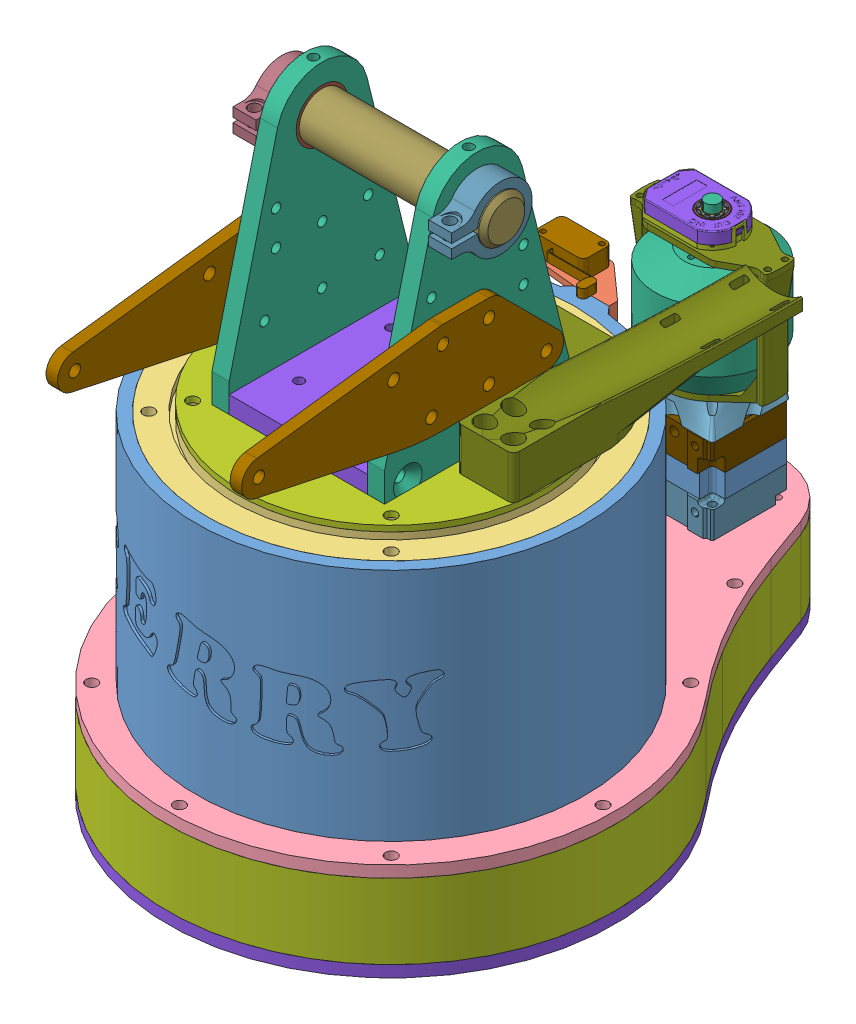
SolidWorks assembly Base, configuration Default. Lengths in mm.
Overall size (246.45 331.62 351.82).
89 component instances, 60 part files, 28 mates.
Components (placement in the parent):
- BotTurretHousing^Base-1: BotTurretHousing^Base [Default] at origin size (214.7 129.6 217.88) (virtual)
- SwitchTripper^Base-2: SwitchTripper^Base [Default] at origin size (28.57 11.52 54.14) (hidden, virtual)
- J1SwitchMount^Base-1: J1SwitchMount^Base [Default] at origin size (48.43 36.2 22.29) (virtual)
- 8in-1: 8in [Default] at (0 58.8 0) size (202 16 202)
- 8in-2: 8in [Default] at (0 -58.8 0) x (1 0 0) z (0 0 -1) size (202 16 202)
- BasePlate^Base-1: BasePlate^Base [Default] at origin size (246.45 6.35 338.52) (virtual)
- BotTurretPlate^Base-1: BotTurretPlate^Base [Default] at origin size (168.46 3.17 168.46) (virtual)
- SideTurretPlate^Base-1: SideTurretPlate^Base [Default] at origin size (9.52 279.65 102.6) (virtual)
- SideTurretPlate^Base-3: SideTurretPlate^Base [Default] x (-1 0 0) z (0 0 -1) size (9.52 279.65 102.6) (virtual)
- TopTurretPlate^Base-1: TopTurretPlate^Base [Default] at origin size (168.46 3.17 168.46) (virtual)
- TopBrace-1: TopBrace [Default] at origin size (76.2 9.53 102.6)
- PivotPlate^Base-1: PivotPlate^Base [Default] at origin size (6.35 50.8 177.8) (virtual)
- PivotPlate^Base-2: PivotPlate^Base [Default] at (101.6 0 0) size (6.35 50.8 177.8) (virtual)
- Keda9to1-1: Keda9to1 [Default] at (0 -48.175 -154.975) x (0 -1 0) z (1 0 0) size (176.96 63 76.93)
  - VersaPlanetary_v2_Single_Stage_10_1_with_BAG.STEP-1: VersaPlanetary_v2_Single_Stage_10_1_with_BAG.STEP [Default] at origin size (163.4 63.52 63.52)
    - 217-2820 Rev1_Public.STEP-1: 217-2820 Rev1_Public.STEP [Default] at (-4.6546 22.225 0) x (0 -0.456494 0.889726) z (-1 0 0) size (39.22 38.88 17.4)
      - 217-2625-100.STEP-1: 217-2625-100.STEP [Default] at origin size (39.22 38.88 12.7)
        - 217-2625-008 Rev1.STEP-1: 217-2625-008 Rev1.STEP [Default] at origin size (34.7 34.7 4.7)
        - 217-2625-010 Rev1.STEP-1: 217-2625-010 Rev1.STEP [Default] at (0 10.193 3.65) x (0.999813 0.019336 0) z (0 0 1) size (4 4 12)
        - 217-2625-010 Rev1.STEP-2: 217-2625-010 Rev1.STEP [Default] at (8.691 -5.3258 3.65) size (4 4 12)
        - 217-2625-010 Rev1.STEP-3: 217-2625-010 Rev1.STEP [Default] at (-8.691 -5.3258 3.65) size (4 4 12)
        - 217-2625-005 Rev1_Planet_Revolving_Follower01.STEP-1: 217-2625-005 Rev1_Planet_Revolving_Follower01.STEP [Default] at (8.691 -5.3258 6.35) x (0.932816 0.360354 0) z (0 0 1) size (16.89 16.89 8)
        - 217-2625-005 Rev1_Planet_Revolving_Follower01.STEP-2: 217-2625-005 Rev1_Planet_Revolving_Follower01.STEP [Default] at (-8.691 -5.3258 6.35) x (-0.932788 -0.360426 0) z (0 0 1) size (16.89 16.89 8)
        - 217-2625-005 Rev1_Planet_Revolving_Follower01.STEP-3: 217-2625-005 Rev1_Planet_Revolving_Follower01.STEP [Default] at (0 10.193 6.35) x (0.893583 0.448898 0) z (0 0 1) size (16.89 16.89 8)
      - 217-2625-007 Rev1_Public.STEP-1: 217-2625-007 Rev1_Public.STEP [Default] at (0 0 6.7) x (0.992772 0.120019 0) z (0 0 1) size (15.27 15.27 12.7)
    - 217-2625-026 Rev1.STEP-1: 217-2625-026 Rev1.STEP [Default] at (-6.5 22.225 0) x (0 -1 0) z (-1 0 0) size (44.45 42 18.12)
    - 217-2742-001 Rev4.STEP-1: 217-2742-001 Rev4.STEP [Default] at (0.2002 22.225 0) x (1 0 0) z (0 -0.092627 0.995701) size (7 28 28)
    - 217-2742-001 Rev4.STEP-2: 217-2742-001 Rev4.STEP [Default] at (8.2002 22.225 0) size (7 28 28)
    - 217-2625-017 Rev1_9714K61.STEP-1: 217-2625-017 Rev1_9714K61.STEP [Default] at (7.42 22.3002 -0.342) x (0 0.56703 0.823697) z (0 -0.823697 0.56703) size (28.51 4.98 27.43)
    - 217-2625-003 Rev1.STEP-1: 217-2625-003 Rev1.STEP [Default] at (7.4478 22.225 0) x (0 -1 0) z (1 0 0) size (17 17 64.11) (hidden)
    - 217-2625-018 Rev1_98541A410.STEP-1: 217-2625-018 Rev1_98541A410.STEP [Default] at (-0.7046 22.225 0) x (1 0 0) z (0 -0.017452 0.999848) size (1 19.6 17.4)
    - 832-1750-Ring-Gear-Screw_SSA0832-0500ZC.STEP-1: 832-1750-Ring-Gear-Screw_SSA0832-0500ZC.STEP [Default] at (-30.7 4.725 -17.5) x (0 0.997447 0.071411) z (0 -0.071411 0.997447) size (6.73 48.51 6.73) (hidden)
    - 832-1750-Ring-Gear-Screw_SSA0832-0500ZC.STEP-2: 832-1750-Ring-Gear-Screw_SSA0832-0500ZC.STEP [Default] at (-30.7 39.725 17.5) x (0 0.005929 0.999982) z (0 -0.999982 0.005929) size (6.73 48.51 6.73) (hidden)
    - 217-2625-025 Rev1.STEP-1: 217-2625-025 Rev1.STEP [Default] at (-23.2 22.225 0) x (0 -1 0) z (-1 0 0) size (44.45 42 18)
    - 217-4649-002 Rev1_SSA0832-0500ZC.STEP-1: 217-4649-002 Rev1_SSA0832-0500ZC.STEP [Default] at (-33.7 4.2645 17.9605) x (0 0.33842 -0.940995) z (0 0.940995 0.33842) size (6.73 16.76 6.73) (hidden)
    - 217-4649-002 Rev1_SSA0832-0500ZC.STEP-2: 217-4649-002 Rev1_SSA0832-0500ZC.STEP [Default] at (-33.7 40.1855 -17.9605) x (0 -0.308932 -0.951084) z (0 0.951084 -0.308932) size (6.73 16.76 6.73) (hidden)
    - 217-4649-006 Rev1_SSA0004-008BA.STEP-1: 217-4649-006 Rev1_SSA0004-008BA.STEP [Default] at (-30.7 22.225 12.5) x (0 0.5 -0.866025) z (0 -0.866025 -0.5) size (7 14 7) (hidden)
    - 217-4649-006 Rev1_SSA0004-008BA.STEP-2: 217-4649-006 Rev1_SSA0004-008BA.STEP [Default] at (-30.7 22.225 -12.5) x (0 -0.5 0.866025) z (0 0.866025 0.5) size (7 14 7) (hidden)
    - 217-2822-003 Rev4.STEP-1: 217-2822-003 Rev4.STEP [Default] at (-32.2 22.225 0) x (0 -1 0) z (-1 0 0) size (42 42 4.8) (hidden)
    - 217-3351 Rev2.STEP-1: 217-3351 Rev2.STEP [Default] at (-33.7 22.225 0) x (0 0 1) z (1 0 0) size (59.07 59.07 84.5) (hidden)
    - 217-2816-001 Rev1.STEP-1: 217-2816-001 Rev1.STEP [Default] at (-6.35 22.225 0) x (0 -1 0) z (1 0 0) size (42 42 14.51)
    - 217-4649-001 Rev1.STEP-1: 217-4649-001 Rev1.STEP [Default] at (-20.046 22.225 0) x (0 -1 0) z (1 0 0) size (18 18 13)
    - 217-4649-007 Rev1_94105A824.STEP-1: 217-4649-007 Rev1_94105A824.STEP [Default] at (-25.521 22.225 -6.7835) x (-0.996104 -0.088191 0) z (0 0 -1) size (4.83 4.83 4.77)
    - 217-2625-011 Rev1.STEP-1: 217-2625-011 Rev1.STEP [Default] at (-24.7818 22.225 0) x (0 0 1) z (0 -1 0) size (8.01 7.5 7.94) (hidden)
  - VersaPlanetary_CIM_Motor_Output_Shaft_Kit_217-2893-1: VersaPlanetary_CIM_Motor_Output_Shaft_Kit_217-2893 [Default] at (7.4478 22.225 0) x (0 0 -1) z (1 0 0) size (17 17 57.85)
  - KedaAdapter^Keda9to1-1: KedaAdapter^Keda9to1 [Default] at origin size (17.82 53.01 53.01) (virtual)
  - 192kvMotorEncoded-1: 192kvMotorEncoded [Default] at (-51.0318 22.225 0) x (0 -1 0) z (0 0 -1) size (63 104.52 76.93)
    - BetterKEDA-1: BetterKEDA [Default] at origin size (63 104.52 63)
    - CUI_DEVICES_AMT102-0048-N2000-S-1: CUI_DEVICES_AMT102-0048-N2000-S [Default] at (0 65.12 0) x (1 0 0) z (0 1 0) size (36.33 46.21 9.2)
      - CUI_DEVICES_AMT102-0048-N2000-S.step-1: CUI_DEVICES_AMT102-0048-N2000-S.step [Default] at origin size (36.33 46.21 9.2)
        - AMT-102-Base-REV-K.step-1: AMT-102-Base-REV-K.step [Default] x (-1 0 0) z (0 0 -1) size (28.78 43.39 9.06)
        - AMT-102-Top-Cover-REV-H.step-1: AMT-102-Top-Cover-REV-H.step [Default] at (0 0 5.23) x (-1 0 0) z (0 0 -1) size (28.6 43.26 6.55)
        - AMT-Sleeve-REV-D_ 2 mm.step-1: AMT-Sleeve-REV-D_ 2 mm.step [Default] at (0 0 -2.42) x (0.999996 0.002864 0) z (0 0 1) size (10.79 10.79 7.8)
        - AMT-Hub-Top-REV-D1.step-1: AMT-Hub-Top-REV-D1.step [Default] at (0 0 2.13) x (0.999996 0.002864 0) z (0 0 1) size (14 14 5.67)
        - AMT-Hub-Bottom-REV-B.step-1: AMT-Hub-Bottom-REV-B.step [Default] at (0 0 2.43) x (0.999998 -0.001942 0) z (0 0 1) size (17.3 17.3 3.2)
        - AMT10X-Shaft-Adaptor-REV-E.step-1: AMT10X-Shaft-Adaptor-REV-E.step [Default] at (0 0 0.03) x (0.999996 0.002864 0) z (0 0 1) size (11.8 11.8 7.8)
        - Receiver-board.step-1: Receiver-board.step [Default] at (72.2834 -20.351 3.03) x (-1 0 0) z (0 0 -1) size (26.5 26.62 0.41)
        - Rotor-board-REV F.step-1: Rotor-board-REV F.step [Default] at (0 0 2.13) x (0.807874 -0.589355 0) z (0 0 1) size (26 26 0.3)
        - Transmitter-board AMT10_AMT-102.step-1: Transmitter-board AMT10_AMT-102.step [Default] at (19.1596 -17.1102 1.22) x (-1 0 0) z (0 0 -1) size (26.63 38.43 4.41)
    - Body^192kvMotorEncoded-1: Body^192kvMotorEncoded [Default] at origin size (53 64.53 76.93) (virtual)
- J1Pulley-1: J1Pulley [Default] at (0 -97.675 0) size (144.9 27.7 144.9)
- 15Tpulley-2: 15Tpulley [Default] at (0 -89.675 -177.2) size (28 28 28)
- J1Belt133T^Base-1: J1Belt133T^Base [Default] at origin size (148.26 15.01 264.1) (virtual)
- TensionPillarJ1-1: TensionPillarJ1 [Default] at (5.0959 -8.1275 -9.5995) size (38.1 25.73 38.1)
  - 98019A228_MIL SPEC. 300 SERIES SS FLAT WASHER-1: 98019A228_MIL SPEC. 300 SERIES SS FLAT WASHER [98019A228] at (20.3041 -73.2587 -110.4505) x (0.972939 0 -0.231063) z (0.231063 0 0.972939) size (9.53 0.71 9.53)
  - 60355K701_BALL BEARING-1: 60355K701_BALL BEARING [60355K701] at (20.3041 -75.7479 -110.4505) x (1 0 0) z (0 1 0) size (15.88 15.88 4.98)
  - Roller^TensionPillarJ1-1: Roller^TensionPillarJ1 [Default] at (-2.0675 -15.5777 2.6827) size (38.1 15 38.1) (virtual)
  - 60355K701_BALL BEARING-2: 60355K701_BALL BEARING [60355K701] at (20.3041 -86.2673 -110.4505) x (1 0 0) z (0 1 0) size (15.88 15.88 4.98)
  - 375spacer-1: 375spacer [92510A777] at (20.3041 -67.785 -110.4505) x (1 0 0) z (0 -1 0) size (15.88 15.88 9.53)
- TensionPillarJ1-2: TensionPillarJ1 [Default] at (-5.0959 -8.1275 -230.5005) x (-1 0 0) z (0 0 -1) size (38.1 25.73 38.1)
  - 98019A228_MIL SPEC. 300 SERIES SS FLAT WASHER-1: 98019A228_MIL SPEC. 300 SERIES SS FLAT WASHER [98019A228] at (20.3041 -73.2587 -110.4505) x (0.972939 0 -0.231063) z (0.231063 0 0.972939) size (9.53 0.71 9.53)
  - 60355K701_BALL BEARING-1: 60355K701_BALL BEARING [60355K701] at (20.3041 -75.7479 -110.4505) x (1 0 0) z (0 1 0) size (15.88 15.88 4.98)
  - Roller^TensionPillarJ1-1: Roller^TensionPillarJ1 [Default] at (-2.0675 -15.5777 2.6827) size (38.1 15 38.1) (virtual)
  - 60355K701_BALL BEARING-2: 60355K701_BALL BEARING [60355K701] at (20.3041 -86.2673 -110.4505) x (1 0 0) z (0 1 0) size (15.88 15.88 4.98)
  - 375spacer-1: 375spacer [92510A777] at (20.3041 -67.785 -110.4505) x (1 0 0) z (0 -1 0) size (15.88 15.88 9.53)
- TensionConnector^Base-1: TensionConnector^Base [Default] at origin size (66.67 5.71 15.88) (virtual)
- Foot^Base-1: Foot^Base [Default] at origin size (246.45 41.27 338.52) (virtual)
- Sole^Base-1: Sole^Base [Default] at origin size (246.45 6.35 338.52) (virtual)
- switch-1: switch [Default] at (-34 69.95 -117.75) x (-1 0 0) z (0 0 -1) size (39.3 10.3 27.5)
- 94459A340_BRASS HEAT-SET INSERT FOR PLASTIC-1: 94459A340_BRASS HEAT-SET INSERT FOR PLASTIC [94459A340] at (0 52.1 -104.175) x (0.708984 0.705225 0) z (-0.705225 0.708984 0) size (7.22 6.55 7.22)
- 94459A340_BRASS HEAT-SET INSERT FOR PLASTIC-2: 94459A340_BRASS HEAT-SET INSERT FOR PLASTIC [94459A340] at (0 39.4 -104.175) x (0.708984 0.705225 0) z (-0.705225 0.708984 0) size (7.22 6.55 7.22)
- 6391K422_OIL-EMBEDDED SLEEVE BEARING-1: 6391K422_OIL-EMBEDDED SLEEVE BEARING [6391K422] at (-44.45 187.45 0) x (0 0 -1) z (1 0 0) size (28.63 28.63 12.7)
- 6061K603_HARDENED PRECISION STEEL SHAFT-1: 6061K603_HARDENED PRECISION STEEL SHAFT [6061K603] at (0 187.45 0) size (127 25.4 25.4)
- 6391K422_OIL-EMBEDDED SLEEVE BEARING-2: 6391K422_OIL-EMBEDDED SLEEVE BEARING [6391K422] at (44.45 187.45 0) x (0 0 -1) z (1 0 0) size (28.63 28.63 12.7)
- SideClamp-1: SideClamp [Default] at origin size (12.7 34.92 44.45)
- MirrorSideClamp-3: MirrorSideClamp [Default] x (-1 0 0) z (0 0 -1) size (12.7 34.92 44.45)
- SwitchTripper^Base-3: SwitchTripper^Base [Default] x (0 0 -1) z (1 0 0) size (28.57 11.52 54.14) (virtual)
- TailGuide^Base-1: TailGuide^Base [Default] at origin (suppressed, hidden, virtual)
- TailGuide2^Base-2: TailGuide2^Base [Default] at origin size (99.54 28.81 160.77) (virtual)
Mates (geometry in assembly coordinates):
- Concentric1: concentric aligned: cylinder of BotTurretHousing^Base-1 through (0 50.8 0) axis (0 -1 0) radius 86.77; cylinder of 8in-1 through (0 64.8 0) axis (0 -1 0) radius 70
- Coincident1: coincident anti-aligned: plane of BotTurretHousing^Base-1 through (0 50.8 0) normal (0 1 0); plane of 8in-1 through (0 50.8 0) normal (0 -1 0)
- Concentric4: concentric anti-aligned: cylinder of BasePlate^Base-1 through (0 -71.15 -177.2) axis (0 1 0) radius 10; cylinder of Keda9to1-1/VersaPlanetary_CIM_Motor_Output_Shaft_Kit_217-2893-1 through (0 -63.3752 -177.2) axis (0 -1 0) radius 8.5
- Concentric5: concentric aligned: cylinder of BasePlate^Base-1 through (17.9605 -71.15 -159.2395) axis (0 1 0) radius 1.9844; cylinder of Keda9to1-1/VersaPlanetary_v2_Single_Stage_10_1_with_BAG.STEP-1/217-2625-026 Rev1.STEP-1 through (17.9605 -48.175 -159.2395) axis (0 1 0) radius 2.0193
- Coincident2: coincident anti-aligned: plane of BasePlate^Base-1 through (0 -64.8 0) normal (0 1 0); plane of Keda9to1-1/VersaPlanetary_v2_Single_Stage_10_1_with_BAG.STEP-1/217-2625-026 Rev1.STEP-1 through (22.225 -64.8 -199.425) normal (0 -1 0)
- Coincident3: coincident aligned: plane of J1Pulley-1 through (0 -97.675 0) normal (0 0 1)
- Coincident4: coincident aligned: plane of J1Pulley-1 through (0 -97.675 0) normal (1 0 0)
- Coincident7: coincident anti-aligned: plane of BotTurretPlate^Base-1 through (0 -69.975 0) normal (0 -1 0); plane of J1Pulley-1 through (0 -69.975 0) normal (0 1 0)
- Concentric6: concentric anti-aligned: cylinder of Keda9to1-1/VersaPlanetary_CIM_Motor_Output_Shaft_Kit_217-2893-1 through (0 -141.9432 -177.2) axis (0 1 0) radius 3.975; cylinder of 15Tpulley-2 through (0 -81.675 -177.2) axis (0 -1 0) radius 4
- Coincident8: coincident anti-aligned: plane of J1Pulley-1 through (0 -97.675 0) normal (0 -1 0); plane of 15Tpulley-2 through (0 -97.675 -177.2) normal (0 1 0)
- Concentric13: concentric anti-aligned: cylinder of BotTurretHousing^Base-1 through (0 52.1 107.3573) axis (0 0 -1) radius 3.2639; cylinder of 94459A340_BRASS HEAT-SET INSERT FOR PLASTIC-1 through (0 52.1 -104.175) axis (0 0 1) radius 3.1623
- Coincident15: coincident aligned: plane of BotTurretHousing^Base-1 through (0 39.4 -110.525) normal (0 0 -1); plane of 94459A340_BRASS HEAT-SET INSERT FOR PLASTIC-1 through (2.5211 54.6078 -110.525) normal (0 0 -1)
- Concentric14: concentric anti-aligned: cylinder of BotTurretHousing^Base-1 through (0 39.4 107.3573) axis (0 0 -1) radius 3.2639; cylinder of 94459A340_BRASS HEAT-SET INSERT FOR PLASTIC-2 through (0 39.4 -104.175) axis (0 0 1) radius 3.1623
- Coincident16: coincident aligned: plane of BotTurretHousing^Base-1 through (0 39.4 -110.525) normal (0 0 -1); plane of 94459A340_BRASS HEAT-SET INSERT FOR PLASTIC-2 through (2.5211 41.9078 -110.525) normal (0 0 -1)
- Parallel1: parallel anti-aligned: plane of BotTurretHousing^Base-1 through (0 64.8 0) normal (0 1 0); plane of switch-1 through (-34 64.8 -117.75) normal (0 -1 0)
- Coincident19: coincident: line of switch-1 through (0 72.45 -109.85) axis (0 -1 0)
- Parallel2: parallel aligned: plane of switch-1 through (-34 75.1 -114.95) normal (0 0 1)
- Tangent1: tangent anti-aligned: cylinder of BotTurretHousing^Base-1 through (0 368.4317 0) axis (0 -1 0) radius 107.35; cylinder of switch-1 through (0 72.45 -109.85) axis (0 -1 0) radius 2.5
- Coincident22: coincident anti-aligned: plane of BotTurretHousing^Base-1 through (0 64.8 0) normal (0 1 0); plane of switch-1 through (-34 64.8 -117.75) normal (0 -1 0)
- Coincident23: coincident aligned: plane of SideTurretPlate^Base-1 through (-38.1 187.45 0) normal (1 0 0); plane of 6391K422_OIL-EMBEDDED SLEEVE BEARING-1 through (-38.1 187.45 0) normal (1 0 0)
- Concentric16: concentric aligned: cylinder of SideTurretPlate^Base-1 through (-38.1 187.45 0) axis (-1 0 0) radius 14.3129; cylinder of 6391K422_OIL-EMBEDDED SLEEVE BEARING-1 through (-38.1 187.45 0) axis (-1 0 0) radius 12.7
- Concentric17: concentric anti-aligned: cylinder of 6391K422_OIL-EMBEDDED SLEEVE BEARING-1 through (-38.1 187.45 0) axis (-1 0 0) radius 12.7; cylinder of 6061K603_HARDENED PRECISION STEEL SHAFT-1 through (-63.5 187.45 0) axis (1 0 0) radius 12.7
- Width1: width anti-aligned: plane of 6061K603_HARDENED PRECISION STEEL SHAFT-1 through (63.5 187.45 0) normal (1 0 0); plane of 6061K603_HARDENED PRECISION STEEL SHAFT-1 through (-63.5 187.45 0) normal (-1 0 0); plane of SideTurretPlate^Base-1 through (-47.625 187.45 0) normal (-1 0 0); plane of SideTurretPlate^Base-3 through (47.625 187.45 0) normal (1 0 0)
- Coincident24: coincident anti-aligned: plane of BasePlate^Base-1 through (0 -71.15 0) normal (0 -1 0); plane of TensionPillarJ1-1/375spacer-1 through (25.4 -71.15 -120.05) normal (0 1 0)
- Concentric18: concentric aligned: circle of BasePlate^Base-1; cylinder of TensionPillarJ1-1/375spacer-1 through (25.4 -80.675 -120.05) axis (0 1 0) radius 7.9375
- Concentric19: concentric aligned: cylinder of TopTurretPlate^Base-1 through (-59.5567 69.975 -7.9375) axis (0 -1 0) radius 2.6035; cylinder of SwitchTripper^Base-3 through (-59.5567 77.9125 -7.9375) axis (0 -1 0) radius 3.175
- Concentric20: concentric aligned: cylinder of TopTurretPlate^Base-1 through (-75.4317 69.975 7.9375) axis (0 -1 0) radius 2.6035; cylinder of SwitchTripper^Base-3 through (-75.4317 77.9125 7.9375) axis (0 -1 0) radius 3.175
- Coincident25: coincident anti-aligned: plane of TopTurretPlate^Base-1 through (0 69.975 0) normal (0 1 0); plane of SwitchTripper^Base-3 through (0 69.975 0) normal (0 -1 0)
